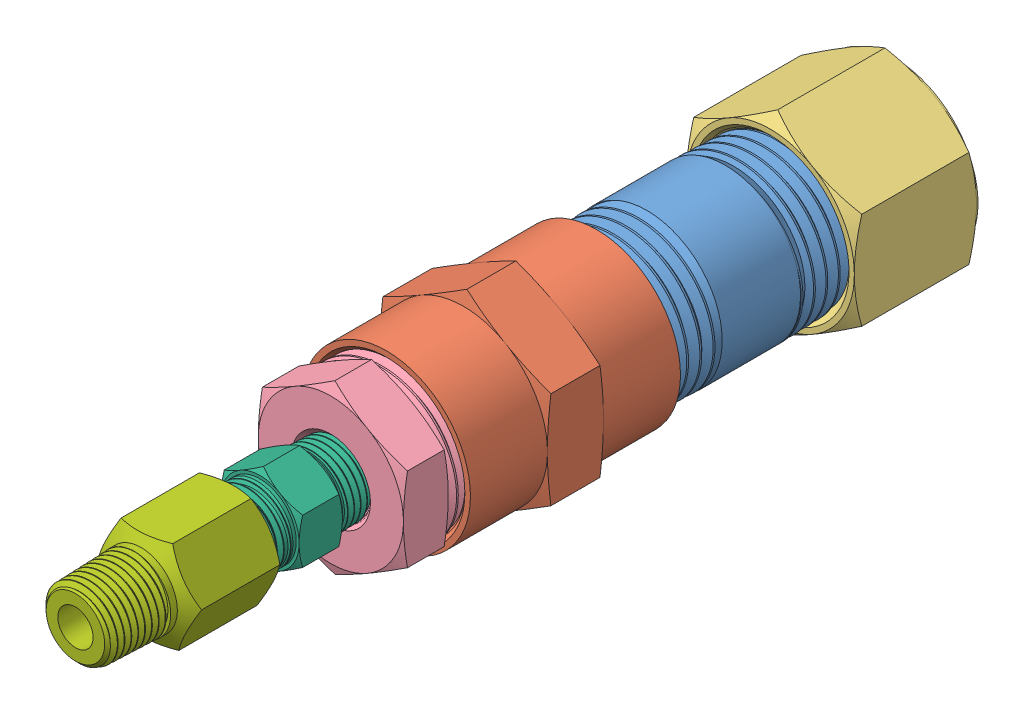
SolidWorks assembly Igniter Cartridge COTS NPT Fittings, configuration Default. Lengths in mm.
Overall size (23.81 27.5 116.32).
7 component instances, 7 part files, 15 mates.
Components (placement in the parent):
- 2155K18_Thick-Wall Aluminum Pipe Nipple-1: 2155K18_Thick-Wall Aluminum Pipe Nipple [2155K18] at origin size (22.44 21.76 51.8)
- 50785K94_High-Pressure Brass Pipe Fitting-1: 50785K94_High-Pressure Brass Pipe Fitting [50785K94] at (0 0 27.5828) size (23.81 27.5 30.36)
- 50785K164_High-Pressure Brass Pipe Fitting-1: 50785K164_High-Pressure Brass Pipe Fitting [50785K164] at (0 0 -11.938) size (23.81 27.5 17.76)
- 4429K421_Low-Pressure Brass Threaded Pipe Fitting-1: 4429K421_Low-Pressure Brass Threaded Pipe Fitting [4429K421] at (0 0 40.0526) x (0 0 -1) z (-1 0 0) size (21.07 23.76 22.01)
- Igniter Estes 13mm-1: Igniter Estes 13mm [Default] at (0 0 -19.912) x (1 0 0) z (0 -1 0) size (13 45 13)
- 5485K21_High-Pressure Brass Pipe Fitting-1: 5485K21_High-Pressure Brass Pipe Fitting [5485K21] at (0 0 57.3246) x (0 0 1) z (-1 0 0) size (24.34 12.83 11.11)
- 50785K25_High-Pressure Brass Pipe Fitting-1: 50785K25_High-Pressure Brass Pipe Fitting [50785K25] at (0 0 75.4221) x (-0.829539 -0.558449 0) z (0 0 -1) size (12.7 14.66 22.71)
Mates (geometry in assembly coordinates):
- Concentric1: concentric aligned: cylinder of 2155K18_Thick-Wall Aluminum Pipe Nipple-1 through (0 0 25.4) axis (0 0 1) radius 10.668; circle of 50785K164_High-Pressure Brass Pipe Fitting-1
- Distance1: distance = 13.462 mm anti-aligned: plane of 50785K164_High-Pressure Brass Pipe Fitting-1 through (-11.9062 20.6222 -11.938) normal (0 0 1); plane of 2155K18_Thick-Wall Aluminum Pipe Nipple-1 through (0 6.9342 -25.4) normal (0 0 -1)
- Distance2: distance = 12.7 mm anti-aligned: plane of 50785K94_High-Pressure Brass Pipe Fitting-1 through (0 11.9062 12.7) normal (0 0 -1); plane of 2155K18_Thick-Wall Aluminum Pipe Nipple-1 through (0 8.576 25.4) normal (0 0 1)
- Concentric2: concentric aligned: cylinder of 2155K18_Thick-Wall Aluminum Pipe Nipple-1 through (0 0 25.4) axis (0 0 1) radius 10.668; cylinder of 50785K94_High-Pressure Brass Pipe Fitting-1 through (0 0 42.4656) axis (0 0 1) radius 11.9062
- Concentric3: concentric aligned: cylinder of 50785K94_High-Pressure Brass Pipe Fitting-1 through (0 0 42.4656) axis (0 0 1) radius 11.9062; cylinder of 4429K421_Low-Pressure Brass Threaded Pipe Fitting-1 through (0 0 29.2673) axis (0 0 1) radius 4.2329
- Distance3: distance = 12.7 mm anti-aligned: plane of 4429K421_Low-Pressure Brass Threaded Pipe Fitting-1 through (0 0 29.7656) normal (0 0 -1); plane of 50785K94_High-Pressure Brass Pipe Fitting-1 through (0 0 42.4656) normal (0 0 1)
- Concentric4: concentric anti-aligned: cylinder of 2155K18_Thick-Wall Aluminum Pipe Nipple-1 through (0 0 25.4) axis (0 0 1) radius 10.668; cylinder of Igniter Estes 13mm-1 through (0 0 25.088) axis (0 0 -1) radius 6.5
- Coincident4: coincident anti-aligned: circle of 2155K18_Thick-Wall Aluminum Pipe Nipple-1; plane of Igniter Estes 13mm-1 through (0 0 25.088) normal (0 0 1)
- Concentric6: concentric anti-aligned: cylinder of 50785K94_High-Pressure Brass Pipe Fitting-1 through (0 0 42.4656) axis (0 0 1) radius 11.9062; cylinder of 5485K21_High-Pressure Brass Pipe Fitting-1 through (0 0 45.2596) axis (0 0 -1) radius 3.175
- Distance5: distance = 5.08 mm anti-aligned: plane of 5485K21_High-Pressure Brass Pipe Fitting-1 through (0 0 45.2596) normal (0 0 -1); plane of 4429K421_Low-Pressure Brass Threaded Pipe Fitting-1 through (10.287 -5.9392 50.3396) normal (0 0 1)
- Concentric7: concentric aligned: cylinder of 5485K21_High-Pressure Brass Pipe Fitting-1 through (0 0 45.2596) axis (0 0 -1) radius 3.175; cylinder of 50785K25_High-Pressure Brass Pipe Fitting (1)-1 through (0 0 77.2382) axis (0 0 -1) radius 2.5019
- Distance6: distance = 5.08 mm anti-aligned: plane of 50785K25_High-Pressure Brass Pipe Fitting (1)-1 through (0 0 64.3096) normal (0 0 -1); plane of 5485K21_High-Pressure Brass Pipe Fitting-1 through (0 0 69.3896) normal (0 0 1)
- Coincident5: coincident aligned: plane of 2155K18_Thick-Wall Aluminum Pipe Nipple-1 through (0 0 0) normal (0 0 1)
- Coincident6: coincident aligned: plane of 2155K18_Thick-Wall Aluminum Pipe Nipple-1 through (0 0 0) normal (0 1 0)
- Coincident7: coincident aligned: plane of 2155K18_Thick-Wall Aluminum Pipe Nipple-1 through (0 0 0) normal (1 0 0)
